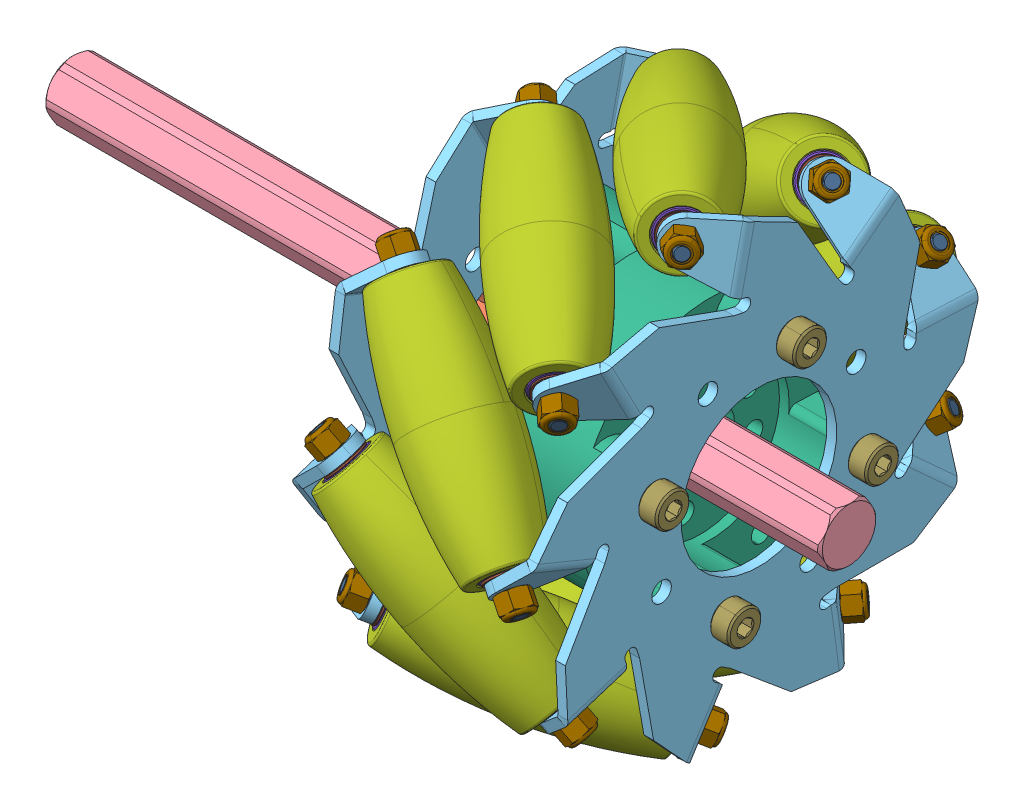
SolidWorks assembly FL Wheel, configuration Default. Lengths in mm.
Overall size (160 142.72 142.72).
96 component instances, 15 part files, 2 mates.
Components (placement in the parent):
- BL Wheel-1: BL Wheel [Default] at (235.3797 -32.5598 108.9761) size (160 36.65 36.37)
  - 12mm ID 1mm Thick Shim.step-1: 12mm ID 1mm Thick Shim.step [Default] at (74.862 410.9212 381.6675) x (0 -0.173258 -0.984876) z (0 0.984876 -0.173258) size (15 1 15)
  - 12mm Axle Collar.STEP-1: 12mm Axle Collar.STEP [Default] at (61.3108 398.0183 360.6125) x (0 -0.536778 -0.843724) z (0 -0.843724 0.536778) size (26 10 26.9)
    - 2910-1026-4012.STEP-1: 2910-1026-4012.STEP [Default] at (-24.6906 18.5512 0.4154) size (26 10 25.98)
    - 2800-0004-0012_90128A207.STEP-1: 2800-0004-0012_90128A207.STEP [Default] at (-16.4406 18.5512 -8.5319) x (0 0.713618 0.700535) z (1 0 0) size (7 7 16.01)
  - 12mm REX 160mm-1: 12mm REX 160mm [Default] at (68.562 410.9212 381.6675) x (0 -0.886725 -0.462297) z (0 -0.462297 0.886725) size (12 160 12.01)
- Mecanum Left Slant With Hyper Hub-1: Mecanum Left Slant With Hyper Hub [Default] at (401.6993 394.2933 385.5104) x (0 0.886214 0.463277) z (0 -0.463277 0.886214) size (119.96 59.77 121.04)
  - Mecanum Left Slant-1: Mecanum Left Slant [Default] at (53.1012 59.4979 77.2081) size (119.96 59.77 121.04)
    - Mecanum 2.STEP-1: Mecanum 2.STEP [Default] at origin size (119.96 59.77 121.04)
      - 3606-0000-0100 Side Plate.STEP-1: 3606-0000-0100 Side Plate.STEP [Default] at (-19.0769 -19.9696 22.3782) size (93.83 10.59 94.33)
      - 3606-0000-0100 Side Plate.STEP-2: 3606-0000-0100 Side Plate.STEP [Default] at (-19.0769 25.889 22.3782) x (1 0 0) z (0 0 -1) size (93.83 10.59 94.33)
      - 3606-XXXX-0100 Wheel Center.STEP-1: 3606-XXXX-0100 Wheel Center.STEP [Default] at (-19.0769 2.9597 22.3782) size (54 46 54)
      - 3606-XXXX-0100 Hi Durability Roller.STEP-1: 3606-XXXX-0100 Hi Durability Roller.STEP [Default] at (5.1459 -41.3984 63.1149) x (0.503693 -0.359647 0.78546) z (-0.696364 -0.707107 0.122788) size (28.35 23.77 47)
      - 3606-XXXX-0100 Roller Bearing.STEP-1: 3606-XXXX-0100 Roller Bearing.STEP [Default] at (-28.4431 -13.6618 64.9271) x (0.292157 -0.123026 0.948424) z (-0.655531 0.696322 0.292257) size (9 4 9)
      - 3606-XXXX-0100 Roller Locknut_90576A102.STEP-1: 3606-XXXX-0100 Roller Locknut_90576A102.STEP [Default] at (-30.184 -15.4296 65.2341) x (-0.521751 0.616262 0.589913) z (0.492801 -0.34673 0.798076) size (5.52 4.01 6.37)
      - 3606-XXXX-0100 Roller Axle.STEP-1: 3606-XXXX-0100 Roller Axle.STEP [Default] at (-12.0786 2.9552 62.0416) x (0.484544 -0.589424 -0.646372) z (0.529428 -0.390615 0.753078) size (4 60.01 4)
      - 3606-XXXX-0100 Roller Shim.STEP-1: 3606-XXXX-0100 Roller Shim.STEP [Default] at (-3.7599 24.6547 102.137) x (-0.324593 0.140076 0.935424) z (0.073634 -0.98223 0.172636) size (7.84 5.87 6.18)
      - 3606-XXXX-0100 Roller Bearing.STEP-2: 3606-XXXX-0100 Roller Bearing.STEP [Default] at (4.286 19.5722 59.1561) x (0.292157 -0.123026 0.948424) z (0.655531 -0.696322 -0.292257) size (9 4 9)
      - 3606-XXXX-0100 Roller Shim.STEP-2: 3606-XXXX-0100 Roller Shim.STEP [Default] at (35.261 37.7727 12.1321) x (-0.012231 -0.482096 -0.876033) z (-0.99905 0.042537 -0.00946) size (7.84 5.87 6.18)
      - 3606-XXXX-0100 Roller Locknut_90576A102.STEP-2: 3606-XXXX-0100 Roller Locknut_90576A102.STEP [Default] at (6.0269 21.34 58.8491) x (0.521751 -0.616262 -0.589913) z (0.492801 -0.34673 0.798076) size (5.52 4.01 6.37)
      - 3606-XXXX-0100 Roller Bearing.STEP-3: 3606-XXXX-0100 Roller Bearing.STEP [Default] at (-24.8203 19.5722 65.569) x (-0.38583 -0.123026 0.91433) z (0.690025 -0.696322 0.197486) size (9 4 9)
      - 3606-XXXX-0100 Roller Bearing.STEP-4: 3606-XXXX-0100 Roller Bearing.STEP [Default] at (-51.2391 19.5722 51.7725) x (-0.883283 -0.123026 0.45241) z (0.401649 -0.696322 0.594822) size (9 4 9)
      - 3606-XXXX-0100 Roller Bearing.STEP-5: 3606-XXXX-0100 Roller Bearing.STEP [Default] at (-62.6089 19.5722 24.2221) x (-0.967438 -0.123026 -0.221197) z (-0.074664 -0.696322 0.713835) size (9 4 9)
      - 3606-XXXX-0100 Roller Bearing.STEP-6: 3606-XXXX-0100 Roller Bearing.STEP [Default] at (-53.6095 19.5722 -4.1911) x (-0.598918 -0.123026 -0.791304) z (-0.51604 -0.696322 0.498837) size (9 4 9)
      - 3606-XXXX-0100 Roller Bearing.STEP-7: 3606-XXXX-0100 Roller Bearing.STEP [Default] at (-28.452 19.5722 -20.1723) x (0.049843 -0.123026 -0.991151) z (-0.715956 -0.696322 0.050427) size (9 4 9)
      - 3606-XXXX-0100 Roller Bearing.STEP-8: 3606-XXXX-0100 Roller Bearing.STEP [Default] at (1.0923 19.5722 -16.2436) x (0.675281 -0.123026 -0.727227) z (-0.580868 -0.696322 -0.421578) size (9 4 9)
      - 3606-XXXX-0100 Roller Bearing.STEP-9: 3606-XXXX-0100 Roller Bearing.STEP [Default] at (21.1992 19.5722 5.7567) x (0.984748 -0.123026 -0.123026) z (-0.173985 -0.696322 -0.696322) size (9 4 9)
      - 3606-XXXX-0100 Roller Bearing.STEP-10: 3606-XXXX-0100 Roller Bearing.STEP [Default] at (22.4605 19.5722 35.5343) x (0.833441 -0.123026 0.538741) z (0.314307 -0.696322 -0.645249) size (9 4 9)
      - 3606-XXXX-0100 Roller Shim.STEP-3: 3606-XXXX-0100 Roller Shim.STEP [Default] at (29.1344 37.7727 49.457) x (0.553733 -0.482096 -0.678942) z (-0.759236 0.042537 -0.649424) size (7.84 5.87 6.18)
      - 3606-XXXX-0100 Roller Shim.STEP-4: 3606-XXXX-0100 Roller Shim.STEP [Default] at (0.4492 37.7727 74.1114) x (0.8606 -0.482096 -0.164167) z (-0.164167 0.042537 -0.985515) size (7.84 5.87 6.18)
      - 3606-XXXX-0100 Roller Shim.STEP-5: 3606-XXXX-0100 Roller Shim.STEP [Default] at (-37.3725 37.7727 74.5592) x (0.764782 -0.482096 0.427424) z (0.507718 0.042537 -0.860473) size (7.84 5.87 6.18)
      - 3606-XXXX-0100 Roller Shim.STEP-6: 3606-XXXX-0100 Roller Shim.STEP [Default] at (-66.6334 37.7727 50.591) x (0.311114 -0.482096 0.819018) z (0.942036 0.042537 -0.332806) size (7.84 5.87 6.18)
      - 3606-XXXX-0100 Roller Shim.STEP-7: 3606-XXXX-0100 Roller Shim.STEP [Default] at (-73.6421 37.7727 13.4217) x (-0.288127 -0.482096 0.827385) z (0.935564 0.042537 0.350585) size (7.84 5.87 6.18)
      - 3606-XXXX-0100 Roller Shim.STEP-8: 3606-XXXX-0100 Roller Shim.STEP [Default] at (-55.1192 37.7727 -19.5568) x (-0.752551 -0.482096 0.448609) z (0.491332 0.042537 0.869933) size (7.84 5.87 6.18)
      - 3606-XXXX-0100 Roller Shim.STEP-9: 3606-XXXX-0100 Roller Shim.STEP [Default] at (-19.7316 37.7727 -32.9134) x (-0.864848 -0.482096 -0.140076) z (-0.1828 0.042537 0.98223) size (7.84 5.87 6.18)
      - 3606-XXXX-0100 Roller Shim.STEP-10: 3606-XXXX-0100 Roller Shim.STEP [Default] at (15.9623 37.7727 -20.3985) x (-0.572473 -0.482096 -0.663218) z (-0.771398 0.042537 0.63493) size (7.84 5.87 6.18)
      - 3606-XXXX-0100 Roller Locknut_90576A102.STEP-3: 3606-XXXX-0100 Roller Locknut_90576A102.STEP [Default] at (-23.2893 21.34 66.4529) x (0.778873 -0.616262 -0.116524) z (-0.135486 -0.34673 0.928128) size (5.52 4.01 6.37)
      - 3606-XXXX-0100 Roller Locknut_90576A102.STEP-4: 3606-XXXX-0100 Roller Locknut_90576A102.STEP [Default] at (-50.6345 21.34 53.4337) x (0.671552 -0.616262 0.411387) z (-0.700378 -0.34673 0.623899) size (5.52 4.01 6.37)
      - 3606-XXXX-0100 Roller Locknut_90576A102.STEP-5: 3606-XXXX-0100 Roller Locknut_90576A102.STEP [Default] at (-63.2135 21.34 25.8832) x (0.250004 -0.616262 0.746806) z (-0.937555 -0.34673 0.02774) size (5.52 4.01 6.37)
      - 3606-XXXX-0100 Roller Locknut_90576A102.STEP-6: 3606-XXXX-0100 Roller Locknut_90576A102.STEP [Default] at (-55.1405 21.34 -3.3072) x (-0.288524 -0.616262 0.732786) z (-0.73604 -0.34673 -0.581399) size (5.52 4.01 6.37)
      - 3606-XXXX-0100 Roller Locknut_90576A102.STEP-7: 3606-XXXX-0100 Roller Locknut_90576A102.STEP [Default] at (-30.1929 21.34 -20.4792) x (-0.692048 -0.616262 0.375887) z (-0.190123 -0.34673 -0.918494) size (5.52 4.01 6.37)
      - 3606-XXXX-0100 Roller Locknut_90576A102.STEP-8: 3606-XXXX-0100 Roller Locknut_90576A102.STEP [Default] at (-0.044 21.34 -17.5977) x (-0.771755 -0.616262 -0.156893) z (0.444754 -0.34673 -0.825816) size (5.52 4.01 6.37)
      - 3606-XXXX-0100 Roller Locknut_90576A102.STEP-9: 3606-XXXX-0100 Roller Locknut_90576A102.STEP [Default] at (21.1992 21.34 3.9889) x (-0.49035 -0.616262 -0.616262) z (0.871526 -0.34673 -0.34673) size (5.52 4.01 6.37)
      - 3606-XXXX-0100 Roller Locknut_90576A102.STEP-10: 3606-XXXX-0100 Roller Locknut_90576A102.STEP [Default] at (23.5968 21.34 34.1802) x (0.020496 -0.616262 -0.787275) z (0.890501 -0.34673 0.294596) size (5.52 4.01 6.37)
      - 3606-XXXX-0100 Roller Bearing.STEP-11: 3606-XXXX-0100 Roller Bearing.STEP [Default] at (-53.6018 -13.6618 48.952) x (-0.38583 -0.123026 0.91433) z (-0.690025 0.696322 -0.197486) size (9 4 9)
      - 3606-XXXX-0100 Roller Bearing.STEP-12: 3606-XXXX-0100 Roller Bearing.STEP [Default] at (-62.6058 -13.6618 20.5428) x (-0.883283 -0.123026 0.45241) z (-0.401649 0.696322 -0.594822) size (9 4 9)
      - 3606-XXXX-0100 Roller Bearing.STEP-13: 3606-XXXX-0100 Roller Bearing.STEP [Default] at (-51.2422 -13.6618 -7.0077) x (-0.967438 -0.123026 -0.221197) z (0.074664 0.696322 -0.713835) size (9 4 9)
      - 3606-XXXX-0100 Roller Bearing.STEP-14: 3606-XXXX-0100 Roller Bearing.STEP [Default] at (-24.828 -13.6618 -20.8081) x (-0.598918 -0.123026 -0.791304) z (0.51604 0.696322 -0.498837) size (9 4 9)
      - 3606-XXXX-0100 Roller Bearing.STEP-15: 3606-XXXX-0100 Roller Bearing.STEP [Default] at (4.2771 -13.6618 -14.4012) x (0.049843 -0.123026 -0.991151) z (0.715956 0.696322 -0.050427) size (9 4 9)
      - 3606-XXXX-0100 Roller Bearing.STEP-16: 3606-XXXX-0100 Roller Bearing.STEP [Default] at (22.4547 -13.6618 9.2152) x (0.675281 -0.123026 -0.727227) z (0.580868 0.696322 0.421578) size (9 4 9)
      - 3606-XXXX-0100 Roller Bearing.STEP-17: 3606-XXXX-0100 Roller Bearing.STEP [Default] at (21.1992 -13.6618 38.9907) x (0.984748 -0.123026 -0.123026) z (0.173985 0.696322 0.696322) size (9 4 9)
      - 3606-XXXX-0100 Roller Bearing.STEP-18: 3606-XXXX-0100 Roller Bearing.STEP [Default] at (1.0981 -13.6618 60.9931) x (0.833441 -0.123026 0.538741) z (-0.314307 0.696322 0.645249) size (9 4 9)
      - 3606-XXXX-0100 Roller Shim.STEP-11: 3606-XXXX-0100 Roller Shim.STEP [Default] at (-58.6113 24.6547 93.3225) x (-0.849932 0.140076 0.507932) z (-0.054562 -0.98223 0.179578) size (7.84 5.87 6.18)
      - 3606-XXXX-0100 Roller Shim.STEP-12: 3606-XXXX-0100 Roller Shim.STEP [Default] at (-94.9642 24.6547 51.3124) x (-0.977578 0.140076 -0.157227) z (-0.157227 -0.98223 0.102493) size (7.84 5.87 6.18)
      - 3606-XXXX-0100 Roller Shim.STEP-13: 3606-XXXX-0100 Roller Shim.STEP [Default] at (-95.8085 24.6547 -4.2363) x (-0.647805 0.140076 -0.748818) z (-0.186324 -0.98223 -0.022549) size (7.84 5.87 6.18)
      - 3606-XXXX-0100 Roller Shim.STEP-14: 3606-XXXX-0100 Roller Shim.STEP [Default] at (-60.7492 24.6547 -47.3318) x (-0.014916 0.140076 -0.990028) z (-0.128238 -0.98223 -0.137041) size (7.84 5.87 6.18)
      - 3606-XXXX-0100 Roller Shim.STEP-15: 3606-XXXX-0100 Roller Shim.STEP [Default] at (-6.191 24.6547 -57.8092) x (0.624951 0.140076 -0.767994) z (-0.010148 -0.98223 -0.187409) size (7.84 5.87 6.18)
      - 3606-XXXX-0100 Roller Shim.STEP-16: 3606-XXXX-0100 Roller Shim.STEP [Default] at (42.3378 24.6547 -30.7661) x (0.972397 0.140076 -0.186606) z (0.11269 -0.98223 -0.150086) size (7.84 5.87 6.18)
      - 3606-XXXX-0100 Roller Shim.STEP-17: 3606-XXXX-0100 Roller Shim.STEP [Default] at (62.13 24.6547 21.1439) x (0.864848 0.140076 0.482096) z (0.1828 -0.98223 -0.042537) size (7.84 5.87 6.18)
      - 3606-XXXX-0100 Roller Shim.STEP-18: 3606-XXXX-0100 Roller Shim.STEP [Default] at (43.9246 24.6547 73.6314) x (0.352626 0.140076 0.925221) z (0.167375 -0.98223 0.084916) size (7.84 5.87 6.18)
      - 3606-XXXX-0100 Roller Axle.STEP-2: 3606-XXXX-0100 Roller Axle.STEP [Default] at (-39.211 2.9552 57.2605) x (0.786662 -0.589424 -0.183691) z (-0.078503 -0.390615 0.917201) size (4 60.01 4)
      - 3606-XXXX-0100 Roller Axle.STEP-3: 3606-XXXX-0100 Roller Axle.STEP [Default] at (-56.9224 2.9552 36.1576) x (0.720693 -0.589424 0.364941) z (-0.649702 -0.390615 0.652156) size (4 60.01 4)
      - 3606-XXXX-0100 Roller Axle.STEP-4: 3606-XXXX-0100 Roller Axle.STEP [Default] at (-56.9255 2.9552 8.6072) x (0.317503 -0.589424 0.742813) z (-0.916899 -0.390615 0.08196) size (4 60.01 4)
      - 3606-XXXX-0100 Roller Axle.STEP-5: 3606-XXXX-0100 Roller Axle.STEP [Default] at (-39.2188 2.9552 -12.4996) x (-0.23425 -0.589424 0.773115) z (-0.755068 -0.390615 -0.526586) size (4 60.01 4)
      - 3606-XXXX-0100 Roller Axle.STEP-6: 3606-XXXX-0100 Roller Axle.STEP [Default] at (-12.0874 2.9552 -17.2867) x (-0.676394 -0.589424 0.441668) z (-0.239932 -0.390615 -0.888737) size (4 60.01 4)
      - 3606-XXXX-0100 Roller Axle.STEP-7: 3606-XXXX-0100 Roller Axle.STEP [Default] at (11.7735 2.9552 -3.5142) x (-0.802047 -0.589424 -0.096441) z (0.38747 -0.390615 -0.835037) size (4 60.01 4)
      - 3606-XXXX-0100 Roller Axle.STEP-8: 3606-XXXX-0100 Roller Axle.STEP [Default] at (21.1992 2.9552 22.3737) x (-0.552412 -0.589424 -0.589424) z (0.833571 -0.390615 -0.390615) size (4 60.01 4)
      - 3606-XXXX-0100 Roller Axle.STEP-9: 3606-XXXX-0100 Roller Axle.STEP [Default] at (11.7793 2.9552 48.2637) x (-0.044298 -0.589424 -0.806609) z (0.889635 -0.390615 0.236581) size (4 60.01 4)
      - 3606-XXXX-0100 Roller Locknut_90576A102.STEP-11: 3606-XXXX-0100 Roller Locknut_90576A102.STEP [Default] at (-55.1327 -15.4296 48.0682) x (-0.778873 0.616262 0.116524) z (-0.135486 -0.34673 0.928128) size (5.52 4.01 6.37)
      - 3606-XXXX-0100 Roller Locknut_90576A102.STEP-12: 3606-XXXX-0100 Roller Locknut_90576A102.STEP [Default] at (-63.2104 -15.4296 18.8816) x (-0.671552 0.616262 -0.411387) z (-0.700378 -0.34673 0.623899) size (5.52 4.01 6.37)
      - 3606-XXXX-0100 Roller Locknut_90576A102.STEP-13: 3606-XXXX-0100 Roller Locknut_90576A102.STEP [Default] at (-50.6375 -15.4296 -8.6688) x (-0.250004 0.616262 -0.746806) z (-0.937555 -0.34673 0.02774) size (5.52 4.01 6.37)
      - 3606-XXXX-0100 Roller Locknut_90576A102.STEP-14: 3606-XXXX-0100 Roller Locknut_90576A102.STEP [Default] at (-23.2971 -15.4296 -21.692) x (0.288524 0.616262 -0.732786) z (-0.73604 -0.34673 -0.581399) size (5.52 4.01 6.37)
      - 3606-XXXX-0100 Roller Locknut_90576A102.STEP-15: 3606-XXXX-0100 Roller Locknut_90576A102.STEP [Default] at (6.018 -15.4296 -14.0943) x (0.692048 0.616262 -0.375887) z (-0.190123 -0.34673 -0.918494) size (5.52 4.01 6.37)
      - 3606-XXXX-0100 Roller Locknut_90576A102.STEP-16: 3606-XXXX-0100 Roller Locknut_90576A102.STEP [Default] at (23.591 -15.4296 10.5694) x (0.771755 0.616262 0.156893) z (0.444754 -0.34673 -0.825816) size (5.52 4.01 6.37)
      - 3606-XXXX-0100 Roller Locknut_90576A102.STEP-17: 3606-XXXX-0100 Roller Locknut_90576A102.STEP [Default] at (21.1992 -15.4296 40.7585) x (0.49035 0.616262 0.616262) z (0.871526 -0.34673 -0.34673) size (5.52 4.01 6.37)
      - 3606-XXXX-0100 Roller Locknut_90576A102.STEP-18: 3606-XXXX-0100 Roller Locknut_90576A102.STEP [Default] at (-0.0382 -15.4296 62.3473) x (-0.020496 0.616262 0.787275) z (0.890501 -0.34673 0.294596) size (5.52 4.01 6.37)
      - 3606-XXXX-0100 Hi Durability Roller.STEP-2: 3606-XXXX-0100 Hi Durability Roller.STEP [Default] at (-26.7061 -41.3984 69.1544) x (-0.119033 -0.359647 0.925465) z (-0.612372 -0.707107 -0.353553) size (28.35 23.77 47)
      - 3606-XXXX-0100 Hi Durability Roller.STEP-3: 3606-XXXX-0100 Hi Durability Roller.STEP [Default] at (-54.9884 -41.3984 53.3069) x (-0.686062 -0.359647 0.632434) z (-0.241845 -0.707107 -0.664463) size (28.35 23.77 47)
      - 3606-XXXX-0100 Hi Durability Roller.STEP-4: 3606-XXXX-0100 Hi Durability Roller.STEP [Default] at (-66.4673 -41.3984 22.9874) x (-0.932075 -0.359647 0.043481) z (0.241845 -0.707107 -0.664463) size (28.35 23.77 47)
      - 3606-XXXX-0100 Hi Durability Roller.STEP-5: 3606-XXXX-0100 Hi Durability Roller.STEP [Default] at (-55.7716 -41.3984 -7.6171) x (-0.74196 -0.359647 -0.565818) z (0.612372 -0.707107 -0.353553) size (28.35 23.77 47)
      - 3606-XXXX-0100 Hi Durability Roller.STEP-6: 3606-XXXX-0100 Hi Durability Roller.STEP [Default] at (-27.9061 -41.3984 -24.1864) x (-0.204673 -0.359647 -0.910364) z (0.696364 -0.707107 0.122788) size (28.35 23.77 47)
      - 3606-XXXX-0100 Hi Durability Roller.STEP-7: 3606-XXXX-0100 Hi Durability Roller.STEP [Default] at (4.0907 -41.3984 -18.9677) x (0.428382 -0.359647 -0.828941) z (0.454519 -0.707107 0.541675) size (28.35 23.77 47)
      - 3606-XXXX-0100 Hi Durability Roller.STEP-8: 3606-XXXX-0100 Hi Durability Roller.STEP [Default] at (25.2472 -41.3984 5.5972) x (0.860993 -0.359647 -0.359647) z (0 -0.707107 0.707107) size (28.35 23.77 47)
      - 3606-XXXX-0100 Hi Durability Roller.STEP-9: 3606-XXXX-0100 Hi Durability Roller.STEP [Default] at (25.6639 -41.3984 38.0142) x (0.890735 -0.359647 0.27793) z (-0.454519 -0.707107 0.541675) size (28.35 23.77 47)
      - 2800-0004-0055_90128A207.STEP-1: 2800-0004-0055_90128A207.STEP [Default] at (-35.0769 32.9597 38.3782) x (0.999526 0 0.030777) z (0 1 0) size (9.08 9.66 59.77)
      - 2800-0004-0055_90128A207.STEP-2: 2800-0004-0055_90128A207.STEP [Default] at (-35.0769 32.9597 6.3782) x (-0.030777 0 0.999526) z (0 1 0) size (9.08 9.66 59.77)
      - 2800-0004-0055_90128A207.STEP-3: 2800-0004-0055_90128A207.STEP [Default] at (-3.0769 32.9597 6.3782) x (-0.999526 0 -0.030777) z (0 1 0) size (9.08 9.66 59.77)
      - 2800-0004-0055_90128A207.STEP-4: 2800-0004-0055_90128A207.STEP [Default] at (-3.0769 32.9597 38.3782) x (0.030777 0 -0.999526) z (0 1 0) size (9.08 9.66 59.77)
      - 2812-0004-0007_90576A103.STEP-1: 2812-0004-0007_90576A103.STEP [Default] at (-35.0769 27.9597 38.3782) x (0.654056 0 0.756446) z (-0.756446 0 0.654056) size (7.02 4.86 8.1)
      - 2812-0004-0007_90576A103.STEP-2: 2812-0004-0007_90576A103.STEP [Default] at (-35.0769 27.9597 6.3782) x (-0.756446 0 0.654056) z (-0.654056 0 -0.756446) size (7.02 4.86 8.1)
      - 2812-0004-0007_90576A103.STEP-3: 2812-0004-0007_90576A103.STEP [Default] at (-3.0769 27.9597 6.3782) x (-0.654056 0 -0.756446) z (0.756446 0 -0.654056) size (7.02 4.86 8.1)
      - 2812-0004-0007_90576A103.STEP-4: 2812-0004-0007_90576A103.STEP [Default] at (-3.0769 27.9597 38.3782) x (0.756446 0 -0.654056) z (0.654056 0 0.756446) size (7.02 4.86 8.1)
  - 12mm Hyper Hub.STEP-1: 12mm Hyper Hub.STEP [Default] at (26.2861 53.0574 117.7049) x (0.999999 0 -0.001105) z (0 1 0) size (26 26 21)
    - 1310-0016-4012.STEP-1: 1310-0016-4012.STEP [Default] at (7.7672 18.1012 8.4002) size (26 26 21)
    - 2800-0004-0014_90128A207.STEP-1: 2800-0004-0014_90128A207.STEP [Default] at (-1.9828 25.8512 24.0002) x (0 0 1) z (-1 0 0) size (7 7 18.01)
    - 2800-0004-0014_90128A207.STEP-2: 2800-0004-0014_90128A207.STEP [Default] at (17.5172 10.3512 24.0002) x (0 0 1) z (1 0 0) size (7 7 18.01)
Mates (geometry in assembly coordinates):
- Coincident1: coincident: plane of BL Wheel-1/12mm Axle Collar.STEP-1/2910-1026-4012.STEP-1 through (320.2417 378.3614 490.6436) normal (1 0 0); plane of Mecanum Left Slant With Hyper Hub-1/12mm Hyper Hub.STEP-1/1310-0016-4012.STEP-1 through (320.2417 378.3139 489.5398) normal (-1 0 0)
- Coincident2: coincident: plane of BL Wheel-1/12mm REX 160mm-1 through (383.9417 372.8665 490.8801) normal (0 -0.999075 0.043001); plane of Mecanum Left Slant With Hyper Hub-1/12mm Hyper Hub.STEP-1/1310-0016-4012.STEP-1 through (320.2417 372.819 489.7763) normal (0 0.999075 -0.043001)
